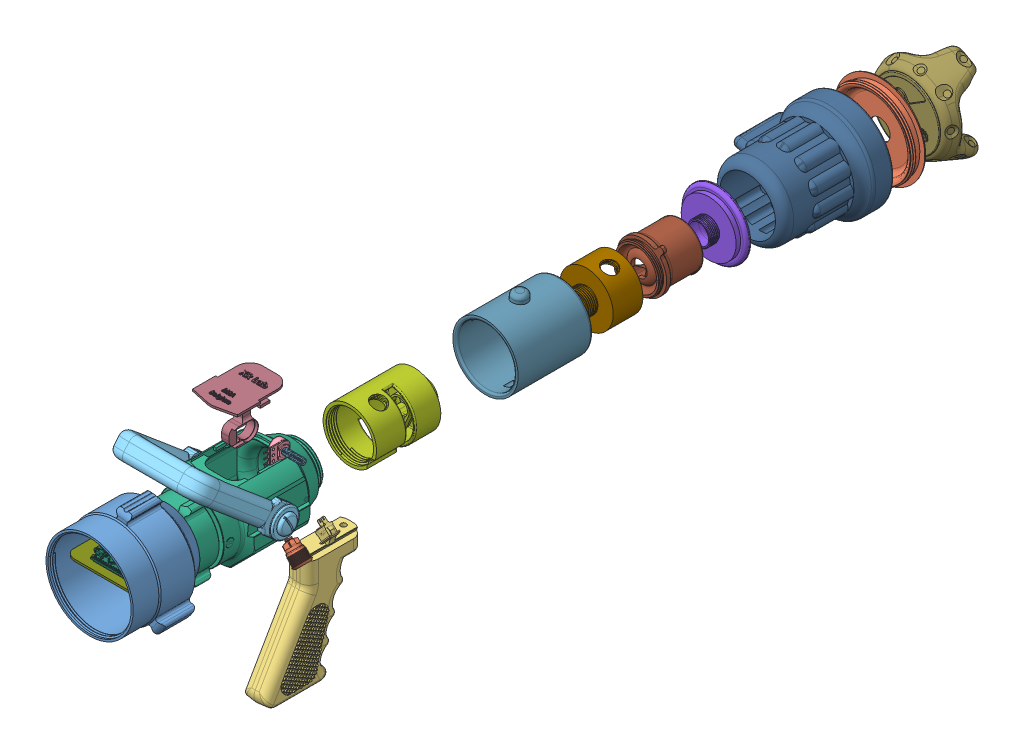
SolidWorks assembly assambled, configuration Défaut. Lengths in mm.
Overall size (135.46 289.51 868.24).
23 component instances, 23 part files, 36 mates.
Components (placement in the parent):
- Back-1: Back [Default] at (3.0126 2.5313 255.8014) x (-0.992574 0.121645 0) z (0 0 -1) size (101.29 101 78.79)
- front-front-1: front-front [Défaut] at (3.0126 2.5313 -237.5001) x (0.758735 -0.6514 0) z (0 0 1) size (91 91 12)
- handle-1: handle [Default] at (2.0156 -37.4687 286.1447) size (28.45 114.3 100.57)
- handle-taraudage-1: handle-taraudage [Défaut] at (8.5223 -14.1498 531.656) x (1 0 0) z (0 -0.181041 -0.983476) size (34.62 19.05 19.05)
- handle-taraudage-main-1: handle-taraudage-main [Défaut] at (8.5223 109.4227 347.5621) x (1 0 0) z (0 -0.666292 0.745691) size (104.46 123.51 41.37)
- main2.1-1: main2.1 [Default] at (3.0126 2.5313 372.0324) size (83.51 83.19 146.64)
- main2.2-1: main2.2 [Default] at (3.0126 2.5313 313.9257) x (0.400709 0.916206 0) z (0 0 1) size (54 54 75)
- main2.3-1: main2.3 [Default] at (3.0126 2.5313 26.187) x (0.980988 0.194066 0) z (0 0 1) size (67.07 67.07 29.26)
- main2.4-1: main2.4 [Default] at (3.0126 2.5313 168.6331) x (0.941038 -0.338301 0) z (0 0 1) size (54 54 40)
- nose-1: nose [Default] at (3.0126 2.5313 -18.3215) x (0.166987 0.985959 0) z (0 0 1) size (126.45 112.17 99.69)
- Nozzle2-1: Nozzle2 [Défaut] at (0.2491 -3.1041 -56.7016) x (0.780961 -0.62458 0) z (0 0 1) size (50 67.44 45.62)
- Support_ViveTracker2xboxControler_Published-1: Support_ViveTracker2xboxControler_Published [Default] at (29.4254 107.676 -230.5656) x (-0.524633 0.851328 0) z (0 0 -1) size (95.05 96.31 42.98)
- top-1: top [Défaut] at (3.6126 100.6259 409.1323) x (0 -1 0) z (1 0 0) size (46.06 60.12 45.2)
- bague-1: bague [Default] at (3.0126 2.5313 176.0157) x (0 0 -1) z (-0.950865 -0.309606 0) size (76 72.82 66)
- arduino nano-1: arduino nano [Default] at (20.3148 3.5813 523.5098) x (-1 0 0) z (0 0 -1) size (45 18.6 18)
- arduino_stack-1: arduino_stack [Default] at (2.5348 1.5813 531.1306) x (0 0 -1) z (1 0 0) size (122 19 78)
- HC-05-1: HC-05 [Default] at (2.5348 -11.8287 469.225) x (0 0 1) z (-1 0 0) size (42.58 6.55 16)
- TTGO32-1: TTGO32 [Default] at (-111.4652 7.5884 496.4142) x (0 0 1) z (1 0 0) size (90 24 28.72)
- vive tripod-1: vive tripod [Défaut] at (3.0126 2.5313 -210.3059) x (0.07548 -0.997147 0) z (0 0 1) size (20 20 40)
- SPST 20mm Pushbutton.step-1: SPST 20mm Pushbutton.step [Default] at (46.6156 -41.0718 392.0324) x (-0.707107 0.707107 0) z (0.262043 0.262043 -0.928799) size (22 17.5 17.5)
- Switch Button-1: Switch Button [Default] at (39.6812 -41.6375 355.9818) x (0.66497 0.74687 0) z (0.74687 -0.66497 0) size (14.91 10.48 19.37)
- Potentiometer_1-2: Potentiometer_1 [Default] at (41.9586 34.6924 371.5557) x (0 0.991445 0.130526) z (1 0 0) size (17 25.82 9)
- PotentiometerB10K-2: PotentiometerB10K [Default] at (41.9586 25.2443 436.2966) x (0 0.20009 -0.979778) z (1 0 0) size (6.01 6.08 20.06)
Mates (geometry in assembly coordinates):
- Distance1: distance = 25 mm: plane of handle-1 through (14.7156 -71.6063 298.3748) normal (1 0 0); plane of main2.1-1 through (39.7156 34.2813 376.7949) normal (1 0 0)
- Coaxiale1: concentric anti-aligned: cylinder of Back-1 through (3.0126 2.5313 538.7694) axis (0 0 -1) radius 45.2437; cylinder of main2.1-1 through (3.0126 2.5313 232.2715) axis (0 0 1) radius 30.9626
- Coaxiale2: concentric anti-aligned: cylinder of main2.1-1 through (3.0126 2.5313 369.6358) axis (0 0 -1) radius 20; cylinder of main2.2-1 through (3.0126 2.5313 205.1648) axis (0 0 1) radius 27
- Coaxiale3: concentric aligned: cylinder of main2.2-1 through (3.0126 2.5313 225.1648) axis (0 0 1) radius 14.5; cylinder of main2.3-1 through (3.0126 2.5313 -81.5214) axis (0 0 1) radius 15
- Coaxiale4: concentric aligned: cylinder of main2.3-1 through (3.0126 2.5313 -81.5214) axis (0 0 1) radius 15; cylinder of main2.4-1 through (3.0126 2.5313 30.9248) axis (0 0 1) radius 27
- Coaxiale5: concentric aligned: cylinder of main2.4-1 through (3.0126 2.5313 30.9248) axis (0 0 1) radius 27; cylinder of Nozzle2-1 through (3.0126 2.5313 -30.1391) axis (0 0 1) radius 23
- Parallèle1: parallel: plane of main2.1-1 through (-4.9874 36.1913 394.3323) normal (0 1 0); plane of top-1 through (3.6126 100.6259 409.1323) normal (0 1 0)
- Coïncidente3: coincident: plane of main2.1-1 through (24.0126 36.1913 424.3323) normal (-1 0 0); plane of top-1 through (24.0126 98.6259 381.3323) normal (1 0 0)
- Coïncidente4: coincident anti-aligned: plane of main2.1-1 through (11.0126 36.1913 381.3323) normal (0 0 1); plane of top-1 through (24.0126 98.6259 381.3323) normal (0 0 -1)
- Coaxiale6: concentric: cylinder of handle-taraudage-main-1 through (45.7855 2.5318 409.333) axis (-1 0 0) radius 14.2875; cylinder of main2.1-1 through (-37.6528 2.5313 409.3323) axis (1 0 0) radius 6.35
- Coaxiale7: concentric aligned: cylinder of nose-1 through (3.0126 2.5313 -196.0299) axis (0 0 1) radius 28; cylinder of Nozzle2-1 through (3.0126 2.5313 -30.1391) axis (0 0 1) radius 23
- Coaxiale9: concentric aligned: cylinder of handle-taraudage-1 through (-24.9565 2.5313 409.3323) axis (-1 0 0) radius 5.75; cylinder of handle-taraudage-main-1 through (60.2914 2.5313 409.3323) axis (-1 0 0) radius 6.5
- Coaxiale10: concentric aligned: cylinder of front-front-1 through (3.0126 2.5313 -225.5001) axis (0 0 -1) radius 40.5; cylinder of nose-1 through (3.0126 2.5313 -201.7181) axis (0 0 -1) radius 36.6713
- Coaxiale11: concentric aligned: cylinder of nose-1 through (3.0126 2.5313 -201.7181) axis (0 0 -1) radius 48.3394; cylinder of Support_ViveTracker2xboxControler_Published-1 through (3.0126 2.5313 -270.519) axis (0 0 -1) radius 3.175
- Coaxiale12: concentric aligned: cylinder of main2.2-1 through (3.0126 2.5313 205.1648) axis (0 0 1) radius 27; cylinder of bague-1 through (3.0126 2.5313 176.0157) axis (0 0 1) radius 29
- Distance2: distance = 40 mm: plane of main2.1-1 through (12.5376 -33.5875 376.7949) normal (0 -1 0); plane of handle-1 through (10.8232 -73.5875 488.7481) normal (0 1 0)
- Coaxiale13: concentric anti-aligned: cylinder of Nozzle2-1 through (3.0126 2.5313 -30.1391) axis (0 0 1) radius 23; cylinder of vive tripod-1 through (3.0126 2.5313 -187.3059) axis (0 0 -1) radius 10
- Coïncidente8: coincident anti-aligned: plane of arduino_stack-1 through (16.6598 -86.4187 531.1306) normal (-1 0 0); plane of TTGO32-1 through (16.6598 3.5813 406.0198) normal (1 0 0)
- Coaxiale14: concentric aligned: cylinder of arduino_stack-1 through (14.5498 6.5813 517.7198) axis (0 -1 0) radius 1.45; cylinder of TTGO32-1 through (14.5498 6.0813 517.7198) axis (0 -1 0) radius 1.5
- Coïncidente9: coincident anti-aligned: plane of arduino_stack-1 through (2.5348 3.5813 531.1306) normal (0 1 0); plane of TTGO32-1 through (2.5348 3.5813 463.0198) normal (0 -1 0)
- Parallèle2: parallel anti-aligned: plane of arduino nano-1 through (-19.0652 5.1813 540.1298) normal (-1 0 0); plane of arduino_stack-1 through (-18.7852 3.5813 531.1306) normal (1 0 0)
- Coïncidente12: coincident anti-aligned: plane of arduino nano-1 through (20.3148 3.5813 523.5098) normal (0 -1 0); plane of arduino_stack-1 through (2.5348 3.5813 531.1306) normal (0 1 0)
- Coaxiale16: concentric aligned: cylinder of arduino nano-1 through (22.8548 5.1813 523.5098) axis (0 -1 0) radius 0.9; cylinder of arduino_stack-1 through (22.8548 6.5813 523.5098) axis (0 -1 0) radius 0.85
- Coïncidente13: coincident anti-aligned: plane of arduino_stack-1 through (10.5348 -7.4187 450.725) normal (-1 0 0); plane of HC-05-1 through (10.5348 -10.5287 487.725) normal (1 0 0)
- Coïncidente14: coincident anti-aligned: plane of arduino_stack-1 through (10.5348 -11.8187 485.725) normal (0 1 0); plane of HC-05-1 through (2.5348 -11.8187 469.225) normal (0 -1 0)
- Coïncidente15: coincident anti-aligned: plane of arduino_stack-1 through (10.5348 -7.4187 487.725) normal (0 0 -1); plane of HC-05-1 through (10.5348 -10.5287 487.725) normal (0 0 1)
- Coïncidente16: coincident: plane of Back-1 through (-36.4874 3.5813 635.3796) normal (1 0 0); plane of arduino_stack-1 through (-36.4874 1.5813 531.1306) normal (-1 0 0)
- Coïncidente17: coincident: plane of Back-1 through (-36.4874 3.5813 635.3796) normal (0 -1 0); plane of arduino_stack-1 through (2.5348 3.5813 531.1306) normal (0 1 0)
- Parallèle4: parallel aligned: plane of handle-1 through (10.8232 -73.5875 488.7481) normal (0 1 0); plane of arduino_stack-1 through (2.5348 3.5813 531.1306) normal (0 1 0)
- Coaxiale17: concentric anti-aligned: cylinder of main2.1-1 through (23.7803 -18.2365 392.0324) axis (0.707107 -0.707107 0) radius 8; cone of SPST 20mm Pushbutton.step-1 through (39.7213 -34.1775 392.0324) axis (-0.707107 0.707107 0)
- Parallèle5: parallel aligned: plane of main2.1-1 through (3.0126 2.5313 359.6358) normal (0 0 -1); plane of Switch Button-1 through (36.1352 -30.3263 352.0318) normal (0 0 -1)
- Coaxiale22: concentric: cylinder of top-1 through (-2.5874 64.6622 409.0376) axis (1 0 0) radius 8.25; cylinder of Potentiometer_1-2 through (42.646 64.6622 409.0376) axis (-1 0 0) radius 8
- Parallèle8: parallel: plane of top-1 through (7.4126 72.2922 409.1323) normal (0 -1 0); plane of Potentiometer_1-2 through (43.646 72.1622 421.0376) normal (0 1 0)
- Coaxiale23: concentric anti-aligned: cylinder of Potentiometer_1-2 through (42.646 64.6622 409.0376) axis (-1 0 0) radius 8; cylinder of PotentiometerB10K-2 through (52.646 64.6622 409.0376) axis (1 0 0) radius 3
- Coïncidente25: coincident anti-aligned: plane of Potentiometer_1-2 through (45.646 64.6622 409.0376) normal (1 0 0); plane of PotentiometerB10K-2 through (45.646 64.7455 409.0435) normal (-1 0 0)
- Coincident1: coincident anti-aligned: plane of handle-taraudage-1 through (-51.4965 2.5313 409.3323) normal (1 0 0); plane of handle-taraudage-main-1 through (-51.4965 2.5318 409.333) normal (-1 0 0)
